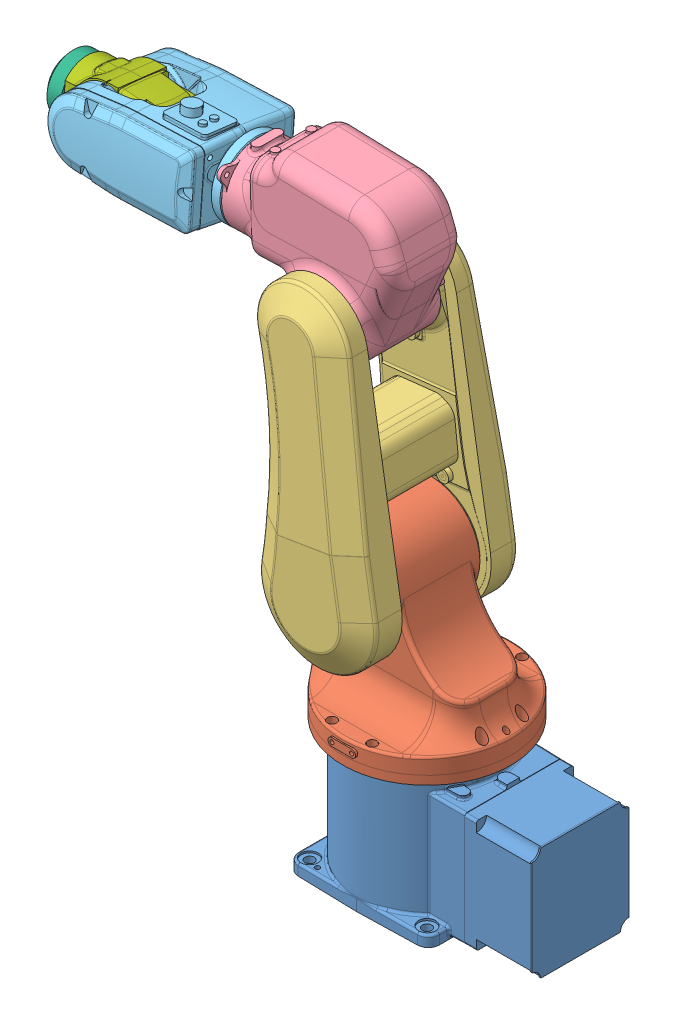
SolidWorks assembly 已解密_ER3A-C60仿真模型, configuration 默认. Lengths in mm.
Overall size (657.7 743.83 223.69).
7 component instances, 7 part files, 21 mates.
Components (placement in the parent):
- Group7^已解密_ER3A-C60仿真模型-1: Group7^已解密_ER3A-C60仿真模型 [默认] at (24.8796 -184.0657 20.4608) x (-1 0 0) z (0 1 0) size (286.41 182.02 166) (virtual)
- Group8^已解密_ER3A-C60仿真模型-1: Group8^已解密_ER3A-C60仿真模型 [默认] at (24.8796 -182.5657 20.4608) x (-1 0 0) z (0 1 0) size (223.55 218 220) (virtual)
- Group9^已解密_ER3A-C60仿真模型-1: Group9^已解密_ER3A-C60仿真模型 [默认] at (79.8368 -171.2794 20.4608) x (-0.99394 -0.109928 0) z (-0.109928 0.99394 0) size (149.57 223.69 407) (virtual)
- Group10^已解密_ER3A-C60仿真模型-1: Group10^已解密_ER3A-C60仿真模型 [默认] at (21.29 -181.2327 20.4608) x (-0.99943 -0.033762 0) z (-0.033762 0.99943 0) size (217.28 107.19 199.19) (virtual)
- Group11^已解密_ER3A-C60仿真模型-1: Group11^已解密_ER3A-C60仿真模型 [默认] at (21.0198 -173.2334 117.7542) x (-0.99943 -0.033762 0) z (-0.033536 0.992749 -0.11543) size (220.5 146.75 108) (virtual)
- 复件 6^已解密_ER3A-C60仿真模型-1: 复件 6^已解密_ER3A-C60仿真模型 [默认] at (-12.9029 800.4244 832.9361) x (-0.99943 -0.033762 0) z (0.004705 -0.139279 -0.990242) size (27.5 70.2 70.2) (virtual)
- 复件 5^已解密_ER3A-C60仿真模型-1: 复件 5^已解密_ER3A-C60仿真模型 [默认] at (19.988 -173.2337 118.0522) x (-0.99943 -0.033762 0) z (-0.033536 0.992749 -0.11543) size (119.98 71.23 82) (virtual)
Mates (geometry in assembly coordinates):
- 同心2: concentric anti-aligned: cylinder of Group10^已解密_ER3A-C60仿真模型-1 through (0.5617 699.8523 45.0534) axis (-0.992859 -0.119296 0) radius 3; cylinder of Group11^已解密_ER3A-C60仿真模型-1 through (-217.993 673.592 45.0534) axis (0.992859 0.119296 0) radius 3
- 同心4: concentric anti-aligned: cylinder of Group8^已解密_ER3A-C60仿真模型-1 through (-97.3762 368.8762 -41.5) axis (0 0 -1) radius 3; cylinder of Group8^已解密_ER3A-C60仿真模型-1 through (-97.3762 368.8762 -66) axis (0 0 1) radius 3
- 同心6: concentric aligned: circle of Group11^已解密_ER3A-C60仿真模型-1; cylinder of 复件 5^已解密_ER3A-C60仿真模型-1 through (-382.0221 653.1898 30.0975) axis (0.003897 -0.115364 -0.993316) radius 27.5
- 同心7: concentric anti-aligned: circle of Group11^已解密_ER3A-C60仿真模型-1; circle of 复件 5^已解密_ER3A-C60仿真模型-1
- 重合1: coincident anti-aligned: plane of 复件 6^已解密_ER3A-C60仿真模型-1 through (-432.875 647.9724 0) normal (0.99943 0.033762 0); plane of 复件 5^已解密_ER3A-C60仿真模型-1 through (-432.875 647.9724 0) normal (-0.99943 -0.033762 0)
- 同心8: concentric aligned: cylinder of 复件 6^已解密_ER3A-C60仿真模型-1 through (-432.875 647.9724 0) axis (-0.99943 -0.033762 0) radius 35.1; circle of 复件 5^已解密_ER3A-C60仿真模型-1
- 同心9: concentric anti-aligned: cylinder of Group9^已解密_ER3A-C60仿真模型-1 through (-79.6806 589.8637 -59.78) axis (0 0 1) radius 34.3; cylinder of Group10^已解密_ER3A-C60仿真模型-1 through (-79.6806 589.8637 -32) axis (0 0 -1) radius 41
- 同心11: concentric anti-aligned: cylinder of Group8^已解密_ER3A-C60仿真模型-1 through (-50 321.5 -46.5) axis (0 0 -1) radius 56; cylinder of Group9^已解密_ER3A-C60仿真模型-1 through (-50 321.5 -85) axis (0 0 1) radius 57
- 同心12: concentric aligned: cylinder of Group7^已解密_ER3A-C60仿真模型-1 through (0 176.5 0) axis (0 1 0) radius 90; cylinder of Group8^已解密_ER3A-C60仿真模型-1 through (0 166.5 0) axis (0 1 0) radius 107.5
- 距离1: distance = 22 mm anti-aligned: plane of Group8^已解密_ER3A-C60仿真模型-1 through (0 170.5 0) normal (0 -1 0); plane of Group7^已解密_ER3A-C60仿真模型-1 through (-33.3876 148.5 49) normal (0 1 0)
- 平行1: parallel aligned: plane of Group7^已解密_ER3A-C60仿真模型-1 through (194 148.5 62) normal (0 0 1); plane of Group8^已解密_ER3A-C60仿真模型-1 through (-50 321.5 52.5) normal (0 0 1)
- 距离2: distance = 5 mm anti-aligned: plane of Group8^已解密_ER3A-C60仿真模型-1 through (-50 321.5 52.5) normal (0 0 1); plane of Group9^已解密_ER3A-C60仿真模型-1 through (-48.1112 318.6906 57.5) normal (0 0 -1)
- 距离3: distance = 9 mm anti-aligned: plane of Group10^已解密_ER3A-C60仿真模型-1 through (-79.6806 589.8637 -49) normal (0 0 -1); plane of Group9^已解密_ER3A-C60仿真模型-1 through (-79.6806 589.8637 -58) normal (0 0 1)
- 同心13: concentric aligned: cylinder of Group10^已解密_ER3A-C60仿真模型-1 through (-63.5889 660.4472 0) axis (-0.99943 -0.033762 0) radius 41; cylinder of Group11^已解密_ER3A-C60仿真模型-1 through (-210.4706 655.4854 0) axis (-0.99943 -0.033762 0) radius 40
- 距离4: distance = 1 mm anti-aligned: plane of Group11^已解密_ER3A-C60仿真模型-1 through (-217.0284 701.5156 -12.9311) normal (0.99943 0.033762 0); plane of Group10^已解密_ER3A-C60仿真模型-1 through (-214.4661 655.2828 -48) normal (-0.99943 -0.033762 0)
- 平行2: parallel aligned: plane of Group10^已解密_ER3A-C60仿真模型-1 through (-51.4527 591.4961 48) normal (0 0 1); plane of 复件 5^已解密_ER3A-C60仿真模型-1
- 重合3: coincident: plane of Group7^已解密_ER3A-C60仿真模型-1 through (0 0 0) normal (0 -1 0); point of assembly
- 同心14: concentric: cylinder of Group7^已解密_ER3A-C60仿真模型-1 through (0 176.5 0) axis (0 1 0) radius 90; point of assembly
- 平行4: parallel anti-aligned: plane of Group7^已解密_ER3A-C60仿真模型-1 through (190 23 -64) normal (0 0 -1); plane of assembly through (0 0 0) normal (0 0 1)
- 平行5: parallel aligned: plane of Group7^已解密_ER3A-C60仿真模型-1 through (-33.3876 148.5 49) normal (0 1 0); plane of assembly through (0 0 0) normal (0 1 0)
- 平行6: parallel aligned: line of Group10^已解密_ER3A-C60仿真模型-1 through (-152.7482 651.2413 48) axis (-0.104464 0.994529 0); line of 复件 6^已解密_ER3A-C60仿真模型-1 through (-435.2253 621.5704 0) axis (-0.104464 0.994529 0)
